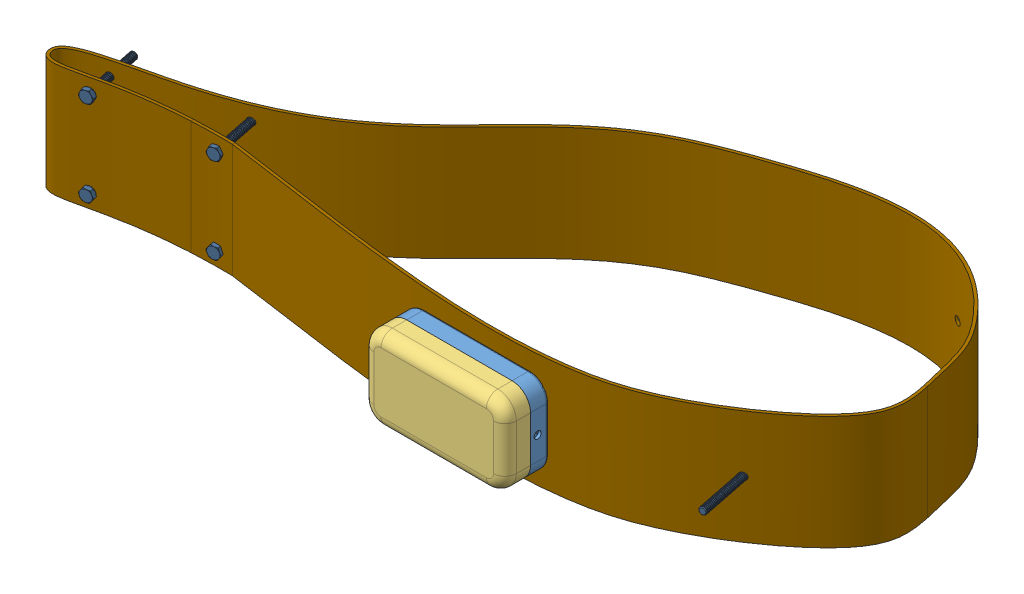
SolidWorks assembly СБ Корпус Peggy Tracker_2, configuration По умолчанию. Lengths in mm.
Overall size (554.96 80.13 309.01).
307 component instances, 82 part files, 17 mates.
Components (placement in the parent):
- Case-03-1: Case-03 [По умолчанию] at (-5.3719 -32.1054 0.6342) size (100 58 14.02)
- Аккумулятор литий-полимерный LP115181-1: Аккумулятор литий-полимерный LP115181 [Default] at (-45.8719 -28.6054 2.6342) size (81 51 11)
- Case-04-1: Case-04 [По умолчанию] at (-5.3719 -32.1054 31.6342) x (-1 0 0) z (0 0 -1) size (100 58 18)
- Печатная плата Peggy Tracker-1: Печатная плата Peggy Tracker [По умолчанию] at (-39.3719 -20.6054 23.0746) x (0 1 0) z (0 0 -1) size (35 62 10.1)
  - Печатная плата Peggy Tracker.step-1: Печатная плата Peggy Tracker.step [Default] at origin size (35 62 10.1)
    - Board.step-1: Board.step [Default] at origin size (35 62 1.56)
      - Open CASCADE STEP translator 6.8 1.1.1.step-1: Open CASCADE STEP translator 6.8 1.1.1.step [Default] at (0 0 -1.5596) size (35 62 1.56)
    - X1.step-1: X1.step [Default] at origin size (28 20 6.7)
      - 6517451856.step-1: 6517451856.step [Default] at (11.15 51.75 6) size (3 3 0.7)
        - Extruded.step-1: Extruded.step [Default] at origin size (3 3 0.7)
      - 6517450176.step-1: 6517450176.step [Default] at (9.1815 45.8445 6) size (6.22 4.19 0.7)
        - Extruded-0.step-1: Extruded-0.step [Default] at origin size (6.22 4.19 0.7)
      - 6517450176.step-2: 6517450176.step [Default] at (9.1815 57.6545 6) size (6.22 4.19 0.7)
        - Extruded-0.step-1: Extruded-0.step [Default] at origin size (6.22 4.19 0.7)
      - 6517449536.step-1: 6517449536.step [Default] at (4.785 51.7495 0) size (2.57 16 6.7)
        - Extruded-1.step-1: Extruded-1.step [Default] at origin size (2.57 16 6.7)
      - 6517449376.step-1: 6517449376.step [Default] at (8.1819 51.7635 6) size (4.22 2.41 0.7)
        - Extruded-2.step-1: Extruded-2.step [Default] at origin size (4.22 2.41 0.7)
      - 6517449056.step-1: 6517449056.step [Default] at (30.8492 51.7495 0) size (1.3 16 6.7)
        - Extruded-3.step-1: Extruded-3.step [Default] at origin size (1.3 16 6.7)
      - 6517448576.step-1: 6517448576.step [Default] at (28.9305 45.5257 6) size (2.54 3.55 0.7)
        - Extruded-4.step-1: Extruded-4.step [Default] at origin size (2.54 3.55 0.7)
      - 6517448256.step-1: 6517448256.step [Default] at (29.4382 51.4325 6) size (1.52 5.71 0.7)
        - Extruded-5.step-1: Extruded-5.step [Default] at origin size (1.52 5.71 0.7)
      - 6517447856.step-1: 6517447856.step [Default] at (18.1354 51.7495 0) size (24.13 16 1)
        - Extruded-6.step-1: Extruded-6.step [Default] at origin size (24.13 16 1)
      - 6517447456.step-1: 6517447456.step [Default] at (18.135 58.925 0) size (24.13 1.65 2.5)
        - Extruded-7.step-1: Extruded-7.step [Default] at origin size (24.13 1.65 2.5)
      - 6517447456.step-2: 6517447456.step [Default] at (18.1356 44.5737 0) size (24.13 1.65 2.5)
        - Extruded-7.step-1: Extruded-7.step [Default] at origin size (24.13 1.65 2.5)
      - 6517447056.step-1: 6517447056.step [Default] at (19.0875 48.7663 0) size (9.53 0.89 2.5)
        - Extruded-8.step-1: Extruded-8.step [Default] at origin size (9.53 0.89 2.5)
      - 6517447056.step-2: 6517447056.step [Default] at (19.0875 54.2273 0) size (9.53 0.89 2.5)
        - Extruded-8.step-1: Extruded-8.step [Default] at origin size (9.53 0.89 2.5)
      - 6517446256.step-1: 6517446256.step [Default] at (28.9302 57.972 6) size (2.54 3.55 0.7)
        - Extruded-9.step-1: Extruded-9.step [Default] at origin size (2.54 3.55 0.7)
      - CircuitWorks-BATT_CR2032.step-1: CircuitWorks-BATT_CR2032.step [Default] at (17.5 51.75 6) x (1 0 0) z (0 1 0) size (20 3.2 20)
    - XW2.step-1: XW2.step [Default] at origin size (2.86 3.01 1.29)
      - IPX.step-1: IPX.step [Default] at (2.0669 38.1281 1.27) x (0 1 0) z (0 0 1) size (3.01 2.86 1.29)
    - XW1.step-1: XW1.step [Default] at origin size (2.86 3.01 1.29)
      - IPX.step-1: IPX.step [Default] at (1.9653 7.4677 1.27) x (0 1 0) z (0 0 1) size (3.01 2.86 1.29)
    - R6.step-1: R6.step [Default] at origin size (0.9 1.7 0.55)
      - 6482559680.step-1: 6482559680.step [Default] at (28.8001 34.2999 0) x (0 -1 0) z (0 0 1) size (1.7 0.9 0.55)
        - Terminal.step-1: Terminal.step [Default] at (-0.85 -0.45 0) size (0.1 0.9 0.55)
          - Open_CASCADE_STEP_translator_6.8_15.2.1.step-1: Open_CASCADE_STEP_translator_6.8_15.2.1.step [Default] at origin size (0.1 0.9 0.55)
        - Terminal.step-2: Terminal.step [Default] at (0.85 0.45 0) x (-1 0 0) z (0 0 1) size (0.1 0.9 0.55)
          - Open_CASCADE_STEP_translator_6.8_15.2.1.step-1: Open_CASCADE_STEP_translator_6.8_15.2.1.step [Default] at origin size (0.1 0.9 0.55)
        - Mid_Body.step-1: Mid_Body.step [Default] at (-0.85 -0.45 0) size (1.59 0.9 0.44)
        - Mark.step-1: Mark.step [Default] at (-0.75 -0.45 0.495) size (1.5 0.9 0.06)
    - X3.step-1: X3.step [Default] at origin size (4.5 5.9 9.4)
      - B2B-PH-K-S(LF)(SN)--3DModel-STEP-56544.step-1: B2B-PH-K-S(LF)(SN)--3DModel-STEP-56544.step [Default] at (32.5449 33.0001 3) x (0 -1 0) z (-1 0 0) size (5.9 9.4 4.5)
    - R5.step-1: R5.step [Default] at origin size (0.95 1.75 0.95)
      - 6482560720.step-1: 6482560720.step [Default] at (27.1578 23.3326 0) x (0 1 0) z (0 0 1) size (1.75 0.95 0.95)
        - Terminal-1.step-1: Terminal-1.step [Default] at (-0.875 -0.475 0) size (0.2 0.95 0.95)
          - Open_CASCADE_STEP_translator_6.8_12.2.1.step-1: Open_CASCADE_STEP_translator_6.8_12.2.1.step [Default] at origin size (0.2 0.95 0.95)
        - Terminal-1.step-2: Terminal-1.step [Default] at (0.875 0.475 0) x (-1 0 0) z (0 0 1) size (0.2 0.95 0.95)
          - Open_CASCADE_STEP_translator_6.8_12.2.1.step-1: Open_CASCADE_STEP_translator_6.8_12.2.1.step [Default] at origin size (0.2 0.95 0.95)
        - Mid_Body-10.step-1: Mid_Body-10.step [Default] at (-0.875 -0.475 0) size (1.56 0.95 0.76)
        - Mark-11.step-1: Mark-11.step [Default] at (-0.675 -0.475 0.855) size (1.35 0.95 0.1)
    - R4.step-1: R4.step [Default] at origin size (0.95 1.75 0.95)
      - 6482560720.step-1: 6482560720.step [Default] at (27.1578 25.8726 0) x (0 1 0) z (0 0 1) size (1.75 0.95 0.95)
        - Terminal-1.step-1: Terminal-1.step [Default] at (-0.875 -0.475 0) size (0.2 0.95 0.95)
          - Open_CASCADE_STEP_translator_6.8_12.2.1.step-1: Open_CASCADE_STEP_translator_6.8_12.2.1.step [Default] at origin size (0.2 0.95 0.95)
        - Terminal-1.step-2: Terminal-1.step [Default] at (0.875 0.475 0) x (-1 0 0) z (0 0 1) size (0.2 0.95 0.95)
          - Open_CASCADE_STEP_translator_6.8_12.2.1.step-1: Open_CASCADE_STEP_translator_6.8_12.2.1.step [Default] at origin size (0.2 0.95 0.95)
        - Mid_Body-10.step-1: Mid_Body-10.step [Default] at (-0.875 -0.475 0) size (1.56 0.95 0.76)
        - Mark-11.step-1: Mark-11.step [Default] at (-0.675 -0.475 0.855) size (1.35 0.95 0.1)
    - R3.step-1: R3.step [Default] at origin size (0.9 1.7 0.55)
      - 6482559680.step-1: 6482559680.step [Default] at (28.8001 31.7999 0) x (0 -1 0) z (0 0 1) size (1.7 0.9 0.55)
        - Terminal.step-1: Terminal.step [Default] at (-0.85 -0.45 0) size (0.1 0.9 0.55)
          - Open_CASCADE_STEP_translator_6.8_15.2.1.step-1: Open_CASCADE_STEP_translator_6.8_15.2.1.step [Default] at origin size (0.1 0.9 0.55)
        - Terminal.step-2: Terminal.step [Default] at (0.85 0.45 0) x (-1 0 0) z (0 0 1) size (0.1 0.9 0.55)
          - Open_CASCADE_STEP_translator_6.8_15.2.1.step-1: Open_CASCADE_STEP_translator_6.8_15.2.1.step [Default] at origin size (0.1 0.9 0.55)
        - Mid_Body.step-1: Mid_Body.step [Default] at (-0.85 -0.45 0) size (1.59 0.9 0.44)
        - Mark.step-1: Mark.step [Default] at (-0.75 -0.45 0.495) size (1.5 0.9 0.06)
    - R2.step-1: R2.step [Default] at origin size (0.9 1.7 0.55)
      - 6482559840.step-1: 6482559840.step [Default] at (24.5109 16.5497 0) x (0 1 0) z (0 0 1) size (1.7 0.9 0.55)
        - Terminal-2.step-1: Terminal-2.step [Default] at (-0.85 -0.45 0) size (0.1 0.9 0.55)
          - Open_CASCADE_STEP_translator_6.8_15.2.1-12.step-1: Open_CASCADE_STEP_translator_6.8_15.2.1-12.step [Default] at origin size (0.1 0.9 0.55)
        - Terminal-2.step-2: Terminal-2.step [Default] at (0.85 0.45 0) x (-1 0 0) z (0 0 1) size (0.1 0.9 0.55)
          - Open_CASCADE_STEP_translator_6.8_15.2.1-12.step-1: Open_CASCADE_STEP_translator_6.8_15.2.1-12.step [Default] at origin size (0.1 0.9 0.55)
        - Mid_Body-13.step-1: Mid_Body-13.step [Default] at (-0.85 -0.45 0) size (1.59 0.9 0.44)
        - Mark-14.step-1: Mark-14.step [Default] at (-0.75 -0.45 0.495) size (1.5 0.9 0.06)
    - R1.step-1: R1.step [Default] at origin size (1.7 0.9 0.55)
      - 6517452256.step-1: 6517452256.step [Default] at (8.2043 34.8489 0) size (1.7 0.9 0.55)
        - Terminal-3.step-1: Terminal-3.step [Default] at (-0.85 -0.45 0) size (0.1 0.9 0.55)
          - Open_CASCADE_STEP_translator_6.8_15.2.1-15.step-1: Open_CASCADE_STEP_translator_6.8_15.2.1-15.step [Default] at origin size (0.1 0.9 0.55)
        - Terminal-3.step-2: Terminal-3.step [Default] at (0.85 0.45 0) x (-1 0 0) z (0 0 1) size (0.1 0.9 0.55)
          - Open_CASCADE_STEP_translator_6.8_15.2.1-15.step-1: Open_CASCADE_STEP_translator_6.8_15.2.1-15.step [Default] at origin size (0.1 0.9 0.55)
        - Mid_Body-16.step-1: Mid_Body-16.step [Default] at (-0.85 -0.45 0) size (1.59 0.9 0.44)
        - Mark-17.step-1: Mark-17.step [Default] at (-0.75 -0.45 0.495) size (1.5 0.9 0.06)
    - L2.step-1: L2.step [Default] at origin size (5.2 5.2 1.8)
      - 6482573440.step-1: 6482573440.step [Default] at (30.1268 13.8076 0.2) x (1 0 0) z (0 -1 0) size (5.2 1.8 5.2)
    - L1.step-1: L1.step [Default] at origin size (0.95 1.75 0.95)
      - 6482561680.step-1: 6482561680.step [Default] at (5.85 37.366 0) x (0 1 0) z (0 0 1) size (1.75 0.95 0.95)
        - Terminal-4.step-1: Terminal-4.step [Default] at (-0.875 -0.475 0) size (1.75 0.95 0.95)
          - Open_CASCADE_STEP_translator_6.8_2.1.1.step-1: Open_CASCADE_STEP_translator_6.8_2.1.1.step [Default] at origin size (0.2 0.95 0.95)
          - Open_CASCADE_STEP_translator_6.8_2.1.2.step-1: Open_CASCADE_STEP_translator_6.8_2.1.2.step [Default] at origin size (0.2 0.95 0.95)
        - Mid_Body-18.step-1: Mid_Body-18.step [Default] at (-0.875 -0.475 0) size (1.35 0.95 0.95)
          - Open_CASCADE_STEP_translator_6.8_2.2.1.step-1: Open_CASCADE_STEP_translator_6.8_2.2.1.step [Default] at origin size (1.35 0.95 0.95)
    - DD2.step-1: DD2.step [Default] at origin size (15 15.5 3.52)
      - 3D_RAK3172.step-1: 3D_RAK3172.step [Default] at (20.536 20.4601 1) x (-1 0 0) z (0 0 1) size (15 15.5 3.52)
        - Board-1.step-1: Board-1.step [Default] at origin size (15 15.5 1.01)
          - Open_CASCADE_STEP_translator_6.8_1.1.1.step-1: Open_CASCADE_STEP_translator_6.8_1.1.1.step [Default] at (0 0 -1.014) size (15 15.5 1.01)
            - Open_CASCADE_STEP_translator_6.8_1.1.1.1.step-1: Open_CASCADE_STEP_translator_6.8_1.1.1.1.step [Default] at origin size (15 15.5 1.01)
        - R11.step-1: R11.step [Default] at origin size (0.6 0.3 0.3)
          - 0201_SMD_Capacitor.step-1: 0201_SMD_Capacitor.step [Default] at (3.4751 6.9342 0.2794) x (-1 0 0) z (0 0 1) size (0.6 0.3 0.3)
        - U2.step-1: U2.step [Default] at origin size (0.99 1.02 0.75)
          - 6590464912.step-1: 6590464912.step [Default] at (5.4483 13.05 0) size (0.99 1.02 0.75)
            - Extruded-19.step-1: Extruded-19.step [Default] at origin size (0.99 1.02 0.75)
        - R4-1.step-1: R4-1.step [Default] at origin size (0.68 0.33 0.34)
          - R0201.step-1: R0201.step [Default] at (3.9176 5.9192 0) x (1 0 0) z (0 -1 0) size (0.68 0.34 0.33)
        - R3-1.step-1: R3-1.step [Default] at origin size (0.33 0.68 0.34)
          - R0201.step-1: R0201.step [Default] at (4.1676 5.6692 0) x (0 1 0) z (1 0 0) size (0.68 0.34 0.33)
        - L2-1.step-1: L2-1.step [Default] at origin size (1.15 0.55 0.41)
          - RES_1005-0402.step-1: RES_1005-0402.step [Default] at (2.2661 6.0198 0) x (1 0 0) z (0 -1 0) size (1.15 0.41 0.55)
        - C10.step-1: C10.step [Default] at origin size (0.6 0.3 0.3)
          - 0201_SMD_Capacitor.step-1: 0201_SMD_Capacitor.step [Default] at (7.1835 13.462 0.2794) x (-1 0 0) z (0 0 1) size (0.6 0.3 0.3)
        - C9.step-1: C9.step [Default] at origin size (0.6 0.3 0.3)
          - 0201_SMD_Capacitor.step-1: 0201_SMD_Capacitor.step [Default] at (7.1835 13.97 0.2794) x (-1 0 0) z (0 0 1) size (0.6 0.3 0.3)
        - C8.step-1: C8.step [Default] at origin size (0.6 0.3 0.3)
          - 0201_SMD_Capacitor.step-1: 0201_SMD_Capacitor.step [Default] at (7.1835 12.954 0.2794) x (-1 0 0) z (0 0 1) size (0.6 0.3 0.3)
        - C7.step-1: C7.step [Default] at origin size (0.6 0.3 0.3)
          - 0201_SMD_Capacitor.step-1: 0201_SMD_Capacitor.step [Default] at (6.0793 11.938 0.2794) x (1 0 0) z (0 0 1) size (0.6 0.3 0.3)
        - C6.step-1: C6.step [Default] at origin size (0.6 0.3 0.3)
          - 0201_SMD_Capacitor.step-1: 0201_SMD_Capacitor.step [Default] at (3.8855 13.5541 0.2794) x (-1 0 0) z (0 0 1) size (0.6 0.3 0.3)
        - CON1.step-1: CON1.step [Default] at origin size (3.4 3.1 1.25)
          - UFL-R-SMD.step-1: UFL-R-SMD.step [Default] at (11.3537 12.7757 0) x (1 0 0) z (0 0 1) size (3.4 3.1 1.25)
            - Part_525.step-1: Part_525.step [Default] at origin size (3 2.6 0.35)
            - Part_739.step-1: Part_739.step [Default] at origin size (2 2 0.9)
            - Part_578.step-1: Part_578.step [Default] at origin size (0.6 0.5 0.1)
            - Part_540.step-1: Part_540.step [Default] at origin size (0.4 1.8 0.1)
            - Part_562.step-1: Part_562.step [Default] at origin size (0.4 1.8 0.1)
            - Part_555.step-1: Part_555.step [Default] at origin size (0.6 0.5 0.1)
        - C4.step-1: C4.step [Default] at origin size (0.6 0.3 0.3)
          - 0201_SMD_Capacitor.step-1: 0201_SMD_Capacitor.step [Default] at (3.7799 9.398 0.2794) x (-1 0 0) z (0 0 1) size (0.6 0.3 0.3)
        - U1.step-1: U1.step [Default] at origin size (7.02 7.02 0.8)
          - QFN48_7x7.step-1: QFN48_7x7.step [Default] at (8.8366 6.9818 0) x (0 1 0) z (1 0 0) size (7.02 0.8 7.02)
        - X1-1.step-1: X1-1.step [Default] at origin size (1.61 2.01 0.71)
          - NT2016SA.step-1: NT2016SA.step [Default] at (1.7496 8.4946 0) x (0 1 0) z (1 0 0) size (2.01 0.71 1.61)
        - C43.step-1: C43.step [Default] at origin size (0.6 0.3 0.3)
          - 0201_SMD_Capacitor.step-1: 0201_SMD_Capacitor.step [Default] at (3.7799 9.9822 0.2794) x (-1 0 0) z (0 0 1) size (0.6 0.3 0.3)
        - C42.step-1: C42.step [Default] at origin size (0.3 0.6 0.3)
          - 0201_SMD_Capacitor.step-1: 0201_SMD_Capacitor.step [Default] at (3.0734 7.9709 0.2794) x (0 -1 0) z (0 0 1) size (0.6 0.3 0.3)
        - R9.step-1: R9.step [Default] at origin size (0.6 0.3 0.3)
          - 0201_SMD_Capacitor.step-1: 0201_SMD_Capacitor.step [Default] at (3.7799 8.8138 0.2794) x (-1 0 0) z (0 0 1) size (0.6 0.3 0.3)
        - C1.step-1: C1.step [Default] at origin size (0.6 0.3 0.3)
          - 0201_SMD_Capacitor.step-1: 0201_SMD_Capacitor.step [Default] at (7.0445 11.557 0.2794) x (1 0 0) z (0 0 1) size (0.6 0.3 0.3)
        - C2.step-1: C2.step [Default] at origin size (0.3 0.6 0.3)
          - 0201_SMD_Capacitor.step-1: 0201_SMD_Capacitor.step [Default] at (7.9756 12.2635 0.2794) x (0 -1 0) z (0 0 1) size (0.6 0.3 0.3)
        - C3.step-1: C3.step [Default] at origin size (0.3 0.6 0.3)
          - 0201_SMD_Capacitor.step-1: 0201_SMD_Capacitor.step [Default] at (2.1844 13.4518 0.2794) x (0 -1 0) z (0 0 1) size (0.6 0.3 0.3)
        - C11.step-1: C11.step [Default] at origin size (0.6 0.3 0.3)
          - 0201_SMD_Capacitor.step-1: 0201_SMD_Capacitor.step [Default] at (1.6623 11.9866 0.2794) x (1 0 0) z (0 0 1) size (0.6 0.3 0.3)
        - C12.step-1: C12.step [Default] at origin size (0.6 0.3 0.3)
          - 0201_SMD_Capacitor.step-1: 0201_SMD_Capacitor.step [Default] at (3.2813 12.573 0.2794) x (1 0 0) z (0 0 1) size (0.6 0.3 0.3)
        - C13.step-1: C13.step [Default] at origin size (0.3 0.6 0.3)
          - 0201_SMD_Capacitor.step-1: 0201_SMD_Capacitor.step [Default] at (4.4958 12.0697 0.2794) x (0 1 0) z (0 0 1) size (0.6 0.3 0.3)
        - C14.step-1: C14.step [Default] at origin size (0.3 0.6 0.3)
          - 0201_SMD_Capacitor.step-1: 0201_SMD_Capacitor.step [Default] at (2.7178 12.6739 0.2794) x (0 -1 0) z (0 0 1) size (0.6 0.3 0.3)
        - C17.step-1: C17.step [Default] at origin size (0.3 0.6 0.3)
          - 0201_SMD_Capacitor.step-1: 0201_SMD_Capacitor.step [Default] at (7.6708 14.4693 0.2794) x (0 -1 0) z (0 0 1) size (0.6 0.3 0.3)
        - C18.step-1: C18.step [Default] at origin size (0.6 0.3 0.3)
          - 0201_SMD_Capacitor.step-1: 0201_SMD_Capacitor.step [Default] at (9.1901 14.1224 0.2794) x (-1 0 0) z (0 0 1) size (0.6 0.3 0.3)
        - C19.step-1: C19.step [Default] at origin size (0.3 0.6 0.3)
          - 0201_SMD_Capacitor.step-1: 0201_SMD_Capacitor.step [Default] at (2.8814 10.8799 0.2794) x (0 1 0) z (0 0 1) size (0.6 0.3 0.3)
        - C22.step-1: C22.step [Default] at origin size (0.3 0.6 0.3)
          - 0201_SMD_Capacitor.step-1: 0201_SMD_Capacitor.step [Default] at (2.0432 11.4801 0.2794) x (0 -1 0) z (0 0 1) size (0.6 0.3 0.3)
        - C21.step-1: C21.step [Default] at origin size (0.3 0.6 0.3)
          - 0201_SMD_Capacitor.step-1: 0201_SMD_Capacitor.step [Default] at (1.5606 11.4801 0.2794) x (0 -1 0) z (0 0 1) size (0.6 0.3 0.3)
        - C23.step-1: C23.step [Default] at origin size (1 0.5 0.5)
          - C0402.step-1: C0402.step [Default] at (8.9644 1.5539 0.254) x (1 0 0) z (0 0 1) size (1 0.5 0.5)
        - C24.step-1: C24.step [Default] at origin size (0.6 0.3 0.3)
          - 0201_SMD_Capacitor.step-1: 0201_SMD_Capacitor.step [Default] at (4.7197 3.8862 0.2794) x (-1 0 0) z (0 0 1) size (0.6 0.3 0.3)
        - C26.step-1: C26.step [Default] at origin size (0.3 0.6 0.3)
          - 0201_SMD_Capacitor.step-1: 0201_SMD_Capacitor.step [Default] at (10.541 2.2265 0.2794) x (0 -1 0) z (0 0 1) size (0.6 0.3 0.3)
        - C44.step-1: C44.step [Default] at origin size (0.6 0.3 0.3)
          - 0201_SMD_Capacitor.step-1: 0201_SMD_Capacitor.step [Default] at (4.7919 9.9822 0.2794) x (-1 0 0) z (0 0 1) size (0.6 0.3 0.3)
        - C29.step-1: C29.step [Default] at origin size (0.6 0.3 0.3)
          - 0201_SMD_Capacitor.step-1: 0201_SMD_Capacitor.step [Default] at (3.9925 7.8486 0.2794) x (1 0 0) z (0 0 1) size (0.6 0.3 0.3)
        - C25.step-1: C25.step [Default] at origin size (0.3 0.6 0.3)
          - 0201_SMD_Capacitor.step-1: 0201_SMD_Capacitor.step [Default] at (10.287 1.6263 0.2794) x (0 1 0) z (0 0 1) size (0.6 0.3 0.3)
        - C31.step-1: C31.step [Default] at origin size (0.6 0.3 0.3)
          - 0201_SMD_Capacitor.step-1: 0201_SMD_Capacitor.step [Default] at (3.9965 7.239 0.2794) x (1 0 0) z (0 0 1) size (0.6 0.3 0.3)
        - C32.step-1: C32.step [Default] at origin size (0.6 0.3 0.3)
          - 0201_SMD_Capacitor.step-1: 0201_SMD_Capacitor.step [Default] at (7.8533 2.3622 0.2794) x (1 0 0) z (0 0 1) size (0.6 0.3 0.3)
        - C33.step-1: C33.step [Default] at origin size (1 0.5 0.5)
          - C0402.step-1: C0402.step [Default] at (5.3048 2.0461 0.254) x (-1 0 0) z (0 0 1) size (1 0.5 0.5)
        - C34.step-1: C34.step [Default] at origin size (0.3 0.6 0.3)
          - 0201_SMD_Capacitor.step-1: 0201_SMD_Capacitor.step [Default] at (4.318 4.2211 0.2794) x (0 1 0) z (0 0 1) size (0.6 0.3 0.3)
        - C35.step-1: C35.step [Default] at origin size (0.6 0.3 0.3)
          - 0201_SMD_Capacitor.step-1: 0201_SMD_Capacitor.step [Default] at (9.0365 2.3622 0.2794) x (1 0 0) z (0 0 1) size (0.6 0.3 0.3)
        - C36.step-1: C36.step [Default] at origin size (0.3 0.6 0.3)
          - 0201_SMD_Capacitor.step-1: 0201_SMD_Capacitor.step [Default] at (13.0302 10.0751 0.2794) x (0 -1 0) z (0 0 1) size (0.6 0.3 0.3)
        - C37.step-1: C37.step [Default] at origin size (0.3 0.6 0.3)
          - 0201_SMD_Capacitor.step-1: 0201_SMD_Capacitor.step [Default] at (3.7338 4.2211 0.2794) x (0 1 0) z (0 0 1) size (0.6 0.3 0.3)
        - C38.step-1: C38.step [Default] at origin size (1 0.5 0.5)
          - C0402.step-1: C0402.step [Default] at (2.3114 4.7323 0.254) x (1 0 0) z (0 0 1) size (1 0.5 0.5)
        - C39.step-1: C39.step [Default] at origin size (0.6 0.3 0.3)
          - 0201_SMD_Capacitor.step-1: 0201_SMD_Capacitor.step [Default] at (4.0593 3.1881 0.2794) x (-1 0 0) z (0 0 1) size (0.6 0.3 0.3)
        - C40.step-1: C40.step [Default] at origin size (0.3 0.6 0.3)
          - 0201_SMD_Capacitor.step-1: 0201_SMD_Capacitor.step [Default] at (3.6576 1.7319 0.2794) x (0 1 0) z (0 0 1) size (0.6 0.3 0.3)
        - L1-1.step-1: L1-1.step [Default] at origin size (0.68 0.33 0.34)
          - R0201.step-1: R0201.step [Default] at (7.8526 11.2014 0) x (-1 0 0) z (0 1 0) size (0.68 0.34 0.33)
        - L3.step-1: L3.step [Default] at origin size (0.33 0.68 0.34)
          - R0201.step-1: R0201.step [Default] at (1.7272 13.1318 0) x (0 -1 0) z (-1 0 0) size (0.68 0.34 0.33)
        - L5.step-1: L5.step [Default] at origin size (0.68 0.33 0.34)
          - R0201.step-1: R0201.step [Default] at (8.0772 13.3096 0) x (-1 0 0) z (0 1 0) size (0.68 0.34 0.33)
        - L6.step-1: L6.step [Default] at origin size (1 0.5 0.5)
          - C0402.step-1: C0402.step [Default] at (5.822 11.0823 0.254) x (1 0 0) z (0 0 1) size (1 0.5 0.5)
        - L7.step-1: L7.step [Default] at origin size (0.68 0.33 0.34)
          - R0201.step-1: R0201.step [Default] at (3.5854 12.1158 0) x (1 0 0) z (0 -1 0) size (0.68 0.34 0.33)
        - L9.step-1: L9.step [Default] at origin size (1.15 0.55 0.41)
          - RES_1005-0402.step-1: RES_1005-0402.step [Default] at (3.9641 11.3538 0) x (-1 0 0) z (0 1 0) size (1.15 0.41 0.55)
        - L20.step-1: L20.step [Default] at origin size (1.6 0.8 0.3)
          - 6559637360.step-1: 6559637360.step [Default] at (12.3698 2.0828 0) x (-1 0 0) z (0 1 0) size (1.6 0.3 0.8)
        - L30.step-1: L30.step [Default] at origin size (1.15 0.55 0.41)
          - RES_1005-0402.step-1: RES_1005-0402.step [Default] at (7.1263 1.8 0) x (-1 0 0) z (0 1 0) size (1.15 0.41 0.55)
        - X2.step-1: X2.step [Default] at origin size (1.2 2 0.61)
          - crystal_rtf2012.step-1: crystal_rtf2012.step [Default] at (2.25 2.8402 0) x (0 1 0) z (1 0 0) size (2 0.61 1.2)
        - R2-1.step-1: R2-1.step [Default] at origin size (0.68 0.33 0.34)
          - R0201.step-1: R0201.step [Default] at (1.9613 10.1854 0) x (1 0 0) z (0 -1 0) size (0.68 0.34 0.33)
        - C5.step-1: C5.step [Default] at origin size (0.6 0.3 0.3)
          - 0201_SMD_Capacitor.step-1: 0201_SMD_Capacitor.step [Default] at (1.8749 6.9342 0.2794) x (-1 0 0) z (0 0 1) size (0.6 0.3 0.3)
        - Free-Models.step-1: Free-Models.step [Default] at origin size (13.4 13.9 2.5)
          - D030A-______.step-1: D030A-______.step [Default] at (2.429 -1.8288 0) size (13.4 13.9 2.5)
    - DD1.step-1: DD1.step [Default] at origin size (9.7 10.1 2.8)
      - 6482566000.step-1: 6482566000.step [Default] at (16.1 34.85 0) x (1 0 0) z (0 0 1) size (9.7 10.1 2.8)
        - Body.step-1: Body.step [Default] at (0 0 0.1) size (9.7 10.1 2.7)
        - Pins.step-1: Pins.step [Default] at origin size (9.56 9.36 0.1)
    - DA1.step-1: DA1.step [Default] at origin size (3 3 1)
      - 6482561360.step-1: 6482561360.step [Default] at (31.2728 20.6686 0) x (0 1 0) z (0 0 1) size (3 3 1)
        - FRAME-DRC0010J.step-1: FRAME-DRC0010J.step [Default] x (1 0 0) z (0 -1 0) size (3 0.2 3)
          - Open CASCADE STEP translator 6.8 1.16.1.2.1.step-1: Open CASCADE STEP translator 6.8 1.16.1.2.1.step [Default] at origin size (1.9 0.2 3)
          - Open CASCADE STEP translator 6.8 1.16.1.2.2.step-1: Open CASCADE STEP translator 6.8 1.16.1.2.2.step [Default] at origin size (0.4 0.2 0.24)
          - Open CASCADE STEP translator 6.8 1.16.1.2.3.step-1: Open CASCADE STEP translator 6.8 1.16.1.2.3.step [Default] at origin size (0.4 0.2 0.24)
          - Open CASCADE STEP translator 6.8 1.16.1.2.4.step-1: Open CASCADE STEP translator 6.8 1.16.1.2.4.step [Default] at origin size (0.4 0.2 0.24)
          - Open CASCADE STEP translator 6.8 1.16.1.2.5.step-1: Open CASCADE STEP translator 6.8 1.16.1.2.5.step [Default] at origin size (0.4 0.2 0.24)
          - Open CASCADE STEP translator 6.8 1.16.1.2.6.step-1: Open CASCADE STEP translator 6.8 1.16.1.2.6.step [Default] at origin size (0.4 0.2 0.24)
          - Open CASCADE STEP translator 6.8 1.16.1.2.7.step-1: Open CASCADE STEP translator 6.8 1.16.1.2.7.step [Default] at origin size (0.4 0.2 0.24)
          - Open CASCADE STEP translator 6.8 1.16.1.2.8.step-1: Open CASCADE STEP translator 6.8 1.16.1.2.8.step [Default] at origin size (0.4 0.2 0.24)
          - Open CASCADE STEP translator 6.8 1.16.1.2.9.step-1: Open CASCADE STEP translator 6.8 1.16.1.2.9.step [Default] at origin size (0.4 0.2 0.24)
          - Open CASCADE STEP translator 6.8 1.16.1.2.10.step-1: Open CASCADE STEP translator 6.8 1.16.1.2.10.step [Default] at origin size (0.4 0.2 0.24)
          - Open CASCADE STEP translator 6.8 1.16.1.2.11.step-1: Open CASCADE STEP translator 6.8 1.16.1.2.11.step [Default] at origin size (0.4 0.2 0.24)
        - BODY-SON.step-1: BODY-SON.step [Default] at (0 0 0.025) x (1 0 0) z (0 -1 0) size (3 0.97 3)
    - C8-1.step-1: C8-1.step [Default] at origin size (1.4 2.15 1.4)
      - 6482573680.step-1: 6482573680.step [Default] at (27.1929 19.9035 0) x (0 -1 0) z (0 0 1) size (2.15 1.4 1.4)
        - Terminal-5.step-1: Terminal-5.step [Default] at (-1.075 -0.7 0) size (2.15 1.4 1.4)
          - Open_CASCADE_STEP_translator_6.8_5.1.1.step-1: Open_CASCADE_STEP_translator_6.8_5.1.1.step [Default] at origin size (0.2 1.4 1.4)
          - Open_CASCADE_STEP_translator_6.8_5.1.2.step-1: Open_CASCADE_STEP_translator_6.8_5.1.2.step [Default] at origin size (0.2 1.4 1.4)
        - Mid_Body-1.step-1: Mid_Body-1.step [Default] at (-1.075 -0.7 0) size (1.75 1.4 1.4)
          - Open_CASCADE_STEP_translator_6.8_5.2.1.step-1: Open_CASCADE_STEP_translator_6.8_5.2.1.step [Default] at origin size (1.75 1.4 1.4)
    - C7-1.step-1: C7-1.step [Default] at origin size (2.1 1.35 1.35)
      - 6482573600.step-1: 6482573600.step [Default] at (31.889 26.8 0) x (1 0 0) z (0 0 1) size (2.1 1.35 1.35)
        - Terminal-6.step-1: Terminal-6.step [Default] at (-1.05 -0.675 0) size (2.1 1.35 1.35)
          - Open_CASCADE_STEP_translator_6.8_24.1.1.step-1: Open_CASCADE_STEP_translator_6.8_24.1.1.step [Default] at origin size (0.2 1.35 1.35)
          - Open_CASCADE_STEP_translator_6.8_24.1.2.step-1: Open_CASCADE_STEP_translator_6.8_24.1.2.step [Default] at origin size (0.2 1.35 1.35)
        - Mid_Body-2.step-1: Mid_Body-2.step [Default] at (-1.05 -0.675 0) size (1.7 1.35 1.35)
          - Open_CASCADE_STEP_translator_6.8_24.2.1.step-1: Open_CASCADE_STEP_translator_6.8_24.2.1.step [Default] at origin size (1.7 1.35 1.35)
    - C6-1.step-1: C6-1.step [Default] at origin size (0.9 1.7 0.9)
      - 6482559520.step-1: 6482559520.step [Default] at (22.727 16.763 0) x (0 -1 0) z (0 0 1) size (1.7 0.9 0.9)
        - Terminal-7.step-1: Terminal-7.step [Default] at (-0.85 -0.45 0) size (1.7 0.9 0.9)
          - Open_CASCADE_STEP_translator_6.8_5.1.1-20.step-1: Open_CASCADE_STEP_translator_6.8_5.1.1-20.step [Default] at origin size (0.2 0.9 0.9)
          - Open_CASCADE_STEP_translator_6.8_5.1.2-21.step-1: Open_CASCADE_STEP_translator_6.8_5.1.2-21.step [Default] at origin size (0.2 0.9 0.9)
        - Mid_Body-3.step-1: Mid_Body-3.step [Default] at (-0.85 -0.45 0) size (1.3 0.9 0.9)
          - Open_CASCADE_STEP_translator_6.8_5.2.1-22.step-1: Open_CASCADE_STEP_translator_6.8_5.2.1-22.step [Default] at origin size (1.3 0.9 0.9)
    - C5-1.step-1: C5-1.step [Default] at origin size (1.35 2.1 1.35)
      - 6482568960.step-1: 6482568960.step [Default] at (24.505 19.939 0) x (0 -1 0) z (0 0 1) size (2.1 1.35 1.35)
        - Terminal-8.step-1: Terminal-8.step [Default] at (-1.05 -0.675 0) size (2.1 1.35 1.35)
          - Open_CASCADE_STEP_translator_6.8_24.1.1-23.step-1: Open_CASCADE_STEP_translator_6.8_24.1.1-23.step [Default] at origin size (0.2 1.35 1.35)
          - Open_CASCADE_STEP_translator_6.8_24.1.2-24.step-1: Open_CASCADE_STEP_translator_6.8_24.1.2-24.step [Default] at origin size (0.2 1.35 1.35)
        - Mid_Body-4.step-1: Mid_Body-4.step [Default] at (-1.05 -0.675 0) size (1.7 1.35 1.35)
          - Open_CASCADE_STEP_translator_6.8_24.2.1-25.step-1: Open_CASCADE_STEP_translator_6.8_24.2.1-25.step [Default] at origin size (1.7 1.35 1.35)
    - C4-1.step-1: C4-1.step [Default] at origin size (0.9 1.7 0.9)
      - 6482559520.step-1: 6482559520.step [Default] at (22.7 19.888 0) x (0 -1 0) z (0 0 1) size (1.7 0.9 0.9)
        - Terminal-7.step-1: Terminal-7.step [Default] at (-0.85 -0.45 0) size (1.7 0.9 0.9)
          - Open_CASCADE_STEP_translator_6.8_5.1.1-20.step-1: Open_CASCADE_STEP_translator_6.8_5.1.1-20.step [Default] at origin size (0.2 0.9 0.9)
          - Open_CASCADE_STEP_translator_6.8_5.1.2-21.step-1: Open_CASCADE_STEP_translator_6.8_5.1.2-21.step [Default] at origin size (0.2 0.9 0.9)
        - Mid_Body-3.step-1: Mid_Body-3.step [Default] at (-0.85 -0.45 0) size (1.3 0.9 0.9)
          - Open_CASCADE_STEP_translator_6.8_5.2.1-22.step-1: Open_CASCADE_STEP_translator_6.8_5.2.1-22.step [Default] at origin size (1.3 0.9 0.9)
    - C3-1.step-1: C3-1.step [Default] at origin size (1.35 2.1 1.35)
      - 6482568960.step-1: 6482568960.step [Default] at (25.7048 39.0008 0) x (0 -1 0) z (0 0 1) size (2.1 1.35 1.35)
        - Terminal-8.step-1: Terminal-8.step [Default] at (-1.05 -0.675 0) size (2.1 1.35 1.35)
          - Open_CASCADE_STEP_translator_6.8_24.1.1-23.step-1: Open_CASCADE_STEP_translator_6.8_24.1.1-23.step [Default] at origin size (0.2 1.35 1.35)
          - Open_CASCADE_STEP_translator_6.8_24.1.2-24.step-1: Open_CASCADE_STEP_translator_6.8_24.1.2-24.step [Default] at origin size (0.2 1.35 1.35)
        - Mid_Body-4.step-1: Mid_Body-4.step [Default] at (-1.05 -0.675 0) size (1.7 1.35 1.35)
          - Open_CASCADE_STEP_translator_6.8_24.2.1-25.step-1: Open_CASCADE_STEP_translator_6.8_24.2.1-25.step [Default] at origin size (1.7 1.35 1.35)
    - C2-1.step-1: C2-1.step [Default] at origin size (0.9 1.7 0.9)
      - 6482561200.step-1: 6482561200.step [Default] at (23.5204 39.0508 0) x (0 1 0) z (0 0 1) size (1.7 0.9 0.9)
        - Terminal-9.step-1: Terminal-9.step [Default] at (-0.85 -0.45 0) size (1.7 0.9 0.9)
          - Open_CASCADE_STEP_translator_6.8_5.1.1-26.step-1: Open_CASCADE_STEP_translator_6.8_5.1.1-26.step [Default] at origin size (0.2 0.9 0.9)
          - Open_CASCADE_STEP_translator_6.8_5.1.2-27.step-1: Open_CASCADE_STEP_translator_6.8_5.1.2-27.step [Default] at origin size (0.2 0.9 0.9)
        - Mid_Body-5.step-1: Mid_Body-5.step [Default] at (-0.85 -0.45 0) size (1.3 0.9 0.9)
          - Open_CASCADE_STEP_translator_6.8_5.2.1-28.step-1: Open_CASCADE_STEP_translator_6.8_5.2.1-28.step [Default] at origin size (1.3 0.9 0.9)
    - C1-1.step-1: C1-1.step [Default] at origin size (0.9 1.7 0.9)
      - 6482559520.step-1: 6482559520.step [Default] at (5.842 33.9488 0) x (0 -1 0) z (0 0 1) size (1.7 0.9 0.9)
        - Terminal-7.step-1: Terminal-7.step [Default] at (-0.85 -0.45 0) size (1.7 0.9 0.9)
          - Open_CASCADE_STEP_translator_6.8_5.1.1-20.step-1: Open_CASCADE_STEP_translator_6.8_5.1.1-20.step [Default] at origin size (0.2 0.9 0.9)
          - Open_CASCADE_STEP_translator_6.8_5.1.2-21.step-1: Open_CASCADE_STEP_translator_6.8_5.1.2-21.step [Default] at origin size (0.2 0.9 0.9)
        - Mid_Body-3.step-1: Mid_Body-3.step [Default] at (-0.85 -0.45 0) size (1.3 0.9 0.9)
          - Open_CASCADE_STEP_translator_6.8_5.2.1-22.step-1: Open_CASCADE_STEP_translator_6.8_5.2.1-22.step [Default] at origin size (1.3 0.9 0.9)
- Ремень-1: Ремень [По умолчанию] at (-216.8921 -3.1054 33.3732) x (-0.980173 0 0.198146) z (0 -1 0) size (523.86 209.36 80.13)
- Hexagon Head Bolt DIN М5-1: Hexagon Head Bolt DIN М5 [DIN 933 - M8X45mm] at (-209.9291 -33.1054 -18.1617) x (-0.198146 0 -0.980173) z (0.892456 0.41349 -0.180414) size (43.5 9.24 8)
- Hexagon Head Bolt DIN М5-2: Hexagon Head Bolt DIN М5 [DIN 933 - M8X45mm] at (-209.9291 26.8946 -18.1617) x (-0.198146 0 -0.980173) z (-0.892456 0.41349 0.180414) size (43.5 9.24 8)
- Hexagon Head Bolt DIN М5-3: Hexagon Head Bolt DIN М5 [DIN 933 - M8X45mm] at (-289.5112 -33.1054 -8.0894) x (-0.198146 0 -0.980173) z (0.892456 0.41349 -0.180414) size (43.5 9.24 8)
- Hexagon Head Bolt DIN М5-4: Hexagon Head Bolt DIN М5 [DIN 933 - M8X45mm] at (-289.5112 26.8946 -8.0894) x (-0.198146 0 -0.980173) z (-0.892456 0.41349 0.180414) size (43.5 9.24 8)
- Hexagon Head Bolt DIN М5-5: Hexagon Head Bolt DIN М5 [DIN 933 - M8X45mm] at (140.2688 -3.1054 -45.4267) x (0.198146 0 0.980173) z (-0.980173 0 0.198146) size (43.5 9.24 8)
Mates (geometry in assembly coordinates):
- Coincident1: coincident anti-aligned: plane of Case-03-1 through (-5.3719 -32.1054 2.6342) normal (0 0 1); plane of Аккумулятор литий-полимерный LP115181-1 through (-45.8719 -28.6054 2.6342) normal (0 0 -1)
- Width1: width anti-aligned: plane of Case-03-1 through (-55.3719 -32.1054 13.6342) normal (-1 0 0); plane of Аккумулятор литий-полимерный LP115181-1 through (44.6281 -13.1054 13.6342) normal (1 0 0); plane of Case-03-1 through (35.1281 -28.6054 13.6342) normal (1 0 0); plane of Аккумулятор литий-полимерный LP115181-1 through (-45.8719 -28.6054 13.6342) normal (-1 0 0)
- Width2: width anti-aligned: plane of Аккумулятор литий-полимерный LP115181-1 through (-45.8719 -28.6054 13.6342) normal (0 -1 0); plane of Case-03-1 through (-45.8719 22.3946 13.6342) normal (0 1 0); plane of Аккумулятор литий-полимерный LP115181-1 through (-55.3719 25.8946 13.6342) normal (0 1 0); plane of Case-03-1 through (44.6281 -32.1054 13.6342) normal (0 -1 0)
- Coincident6: coincident anti-aligned: plane of Case-03-1 through (-5.3719 -32.1054 13.6342) normal (0 0 1); plane of Case-04-1 through (-5.3719 -32.1054 13.6342) normal (0 0 -1)
- Coincident3: coincident aligned: plane of Case-03-1 through (-55.3719 -32.1054 13.6342) normal (-1 0 0); plane of Case-04-1 through (-55.3719 -13.1054 63.6342) normal (-1 0 0)
- Coincident4: coincident aligned: plane of Case-03-1 through (-55.3719 25.8946 13.6342) normal (0 1 0); plane of Case-04-1 through (44.6281 25.8946 63.6342) normal (0 1 0)
- Coincident5: coincident anti-aligned: plane of Case-04-1 through (23.6281 12.3946 74.6342) normal (0 0 -1); plane of Печатная плата Peggy Tracker-1/Печатная плата Peggy Tracker.step-1/Board.step-1/Open CASCADE STEP translator 6.8 1.1.1.step-1 through (-36.3719 -20.6054 74.6342) normal (0 0 1)
- Concentric1: concentric aligned: cylinder of Case-04-1 through (23.6281 12.3946 74.6342) axis (0 0 1) radius 1.25; cylinder of Печатная плата Peggy Tracker-1/Печатная плата Peggy Tracker.step-1/Board.step-1/Open CASCADE STEP translator 6.8 1.1.1.step-1 through (23.6281 12.3946 74.6342) axis (0 0 1) radius 1.25
- Concentric2: concentric aligned: cylinder of Case-04-1 through (-34.3719 12.3946 74.6342) axis (0 0 1) radius 1.25; cylinder of Печатная плата Peggy Tracker-1/Печатная плата Peggy Tracker.step-1/Board.step-1/Open CASCADE STEP translator 6.8 1.1.1.step-1 through (-34.3719 12.3946 74.6342) axis (0 0 1) radius 1.25
- Width3: width aligned: plane of Ремень-1 through (-179.3182 -43.1054 -20.5126) normal (0 -1 0); plane of Case-03-1 through (-179.3182 36.8946 -20.5126) normal (0 1 0); plane of Ремень-1 through (44.6281 -32.1054 13.6342) normal (0 -1 0); plane of Case-03-1 through (-55.3719 25.8946 13.6342) normal (0 1 0)
- Tangent2: tangent anti-aligned: plane of Case-03-1 through (-5.3719 -32.1054 0.6342) normal (0 0 -1); face of ?
- Concentric3: concentric aligned: cylinder of Ремень-1 through (-203.9825 -33.1054 -87.0852) axis (0.200475 0 0.979699) radius 2.65; circle of Hexagon Head Bolt DIN М5-1
- Tangent3: tangent: edge_curve of ?; circle of ?
- Concentric4: concentric aligned: cylinder of Ремень-1 through (-282.3584 -33.1054 -71.0472) axis (0.200475 0 0.979699) radius 2.65; circle of Hexagon Head Bolt DIN М5-3
- Tangent4: tangent: edge_curve of ?; circle of ?
- Concentric5: concentric anti-aligned: cylinder of Ремень-1 through (153.4336 -3.1054 -79.586) axis (0.200475 0 0.979699) radius 2.65; circle of Hexagon Head Bolt DIN М5-5
- Tangent5: tangent: edge_curve of ?; circle of ?
